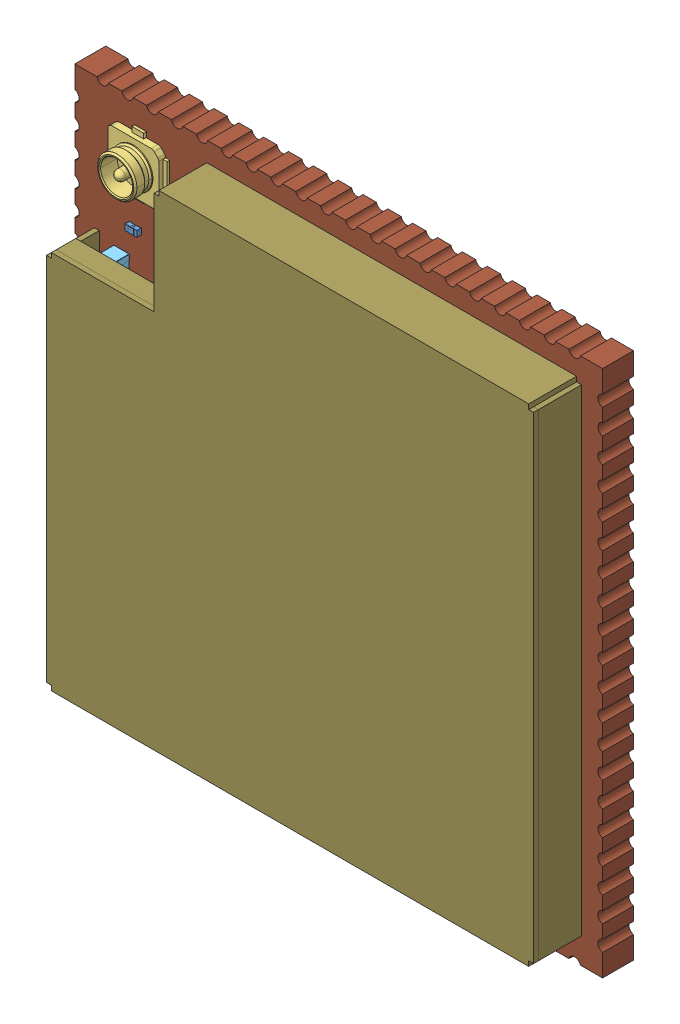
SolidWorks assembly 装配体1, configuration 默认. Lengths in mm.
Overall size (26.97 26.97 4.04).
150 component instances, 12 part files, 3 mates.
Components (placement in the parent):
- 3D_ESP32-P4-Core_2025-12-02-1: 3D_ESP32-P4-Core_2025-12-02 [默认] at (-120.883 -11.4499 -1.4231) size (26.97 26.97 2.85)
  - 3D_ESP32-P4-Core_2025-12-02.step-1: 3D_ESP32-P4-Core_2025-12-02.step [默认] at origin size (26.97 26.97 2.85)
    - R1~R0201~R0201_L0.6-W0.3-H0.3~E7ic.step-1: R1~R0201~R0201_L0.6-W0.3-H0.3~E7ic.step [默认] at (21.717 19.558 1.5862) x (0 -1 0) z (0 0 1) size (0.6 0.3 0.24)
      - R0201~R0201_L0.6-W0.3-H0.3~E7ic.step-1: R0201~R0201_L0.6-W0.3-H0.3~E7ic.step [默认] at origin size (0.6 0.3 0.24)
    - R1~R0201~R0201_L0.6-W0.3-H0.3~E7ic.step-2: R1~R0201~R0201_L0.6-W0.3-H0.3~E7ic.step [默认] at (21.463 20.7645 1.5862) size (0.6 0.3 0.24)
      - R0201~R0201_L0.6-W0.3-H0.3~E7ic.step-1: R0201~R0201_L0.6-W0.3-H0.3~E7ic.step [默认] at origin size (0.6 0.3 0.24)
    - R1~R0201~R0201_L0.6-W0.3-H0.3~E7ic.step-3: R1~R0201~R0201_L0.6-W0.3-H0.3~E7ic.step [默认] at (20.193 4.064 1.5862) x (0 -1 0) z (0 0 1) size (0.6 0.3 0.24)
      - R0201~R0201_L0.6-W0.3-H0.3~E7ic.step-1: R0201~R0201_L0.6-W0.3-H0.3~E7ic.step [默认] at origin size (0.6 0.3 0.24)
    - R1~R0201~R0201_L0.6-W0.3-H0.3~E7ic.step-4: R1~R0201~R0201_L0.6-W0.3-H0.3~E7ic.step [默认] at (14.351 4.1275 1.5862) x (0 -1 0) z (0 0 1) size (0.6 0.3 0.24)
      - R0201~R0201_L0.6-W0.3-H0.3~E7ic.step-1: R0201~R0201_L0.6-W0.3-H0.3~E7ic.step [默认] at origin size (0.6 0.3 0.24)
    - R1~R0201~R0201_L0.6-W0.3-H0.3~E7ic.step-5: R1~R0201~R0201_L0.6-W0.3-H0.3~E7ic.step [默认] at (9.652 15.748 1.5862) size (0.6 0.3 0.24)
      - R0201~R0201_L0.6-W0.3-H0.3~E7ic.step-1: R0201~R0201_L0.6-W0.3-H0.3~E7ic.step [默认] at origin size (0.6 0.3 0.24)
    - R1~R0201~R0201_L0.6-W0.3-H0.3~E7ic.step-6: R1~R0201~R0201_L0.6-W0.3-H0.3~E7ic.step [默认] at (9.652 14.859 1.5862) size (0.6 0.3 0.24)
      - R0201~R0201_L0.6-W0.3-H0.3~E7ic.step-1: R0201~R0201_L0.6-W0.3-H0.3~E7ic.step [默认] at origin size (0.6 0.3 0.24)
    - R1~R0201~R0201_L0.6-W0.3-H0.3~E7ic.step-7: R1~R0201~R0201_L0.6-W0.3-H0.3~E7ic.step [默认] at (9.652 13.97 1.5862) size (0.6 0.3 0.24)
      - R0201~R0201_L0.6-W0.3-H0.3~E7ic.step-1: R0201~R0201_L0.6-W0.3-H0.3~E7ic.step [默认] at origin size (0.6 0.3 0.24)
    - R1~R0201~R0201_L0.6-W0.3-H0.3~E7ic.step-8: R1~R0201~R0201_L0.6-W0.3-H0.3~E7ic.step [默认] at (9.652 13.081 1.5862) size (0.6 0.3 0.24)
      - R0201~R0201_L0.6-W0.3-H0.3~E7ic.step-1: R0201~R0201_L0.6-W0.3-H0.3~E7ic.step [默认] at origin size (0.6 0.3 0.24)
    - R1~R0201~R0201_L0.6-W0.3-H0.3~E7ic.step-9: R1~R0201~R0201_L0.6-W0.3-H0.3~E7ic.step [默认] at (10.033 9.144 1.5862) x (0 -1 0) z (0 0 1) size (0.6 0.3 0.24)
      - R0201~R0201_L0.6-W0.3-H0.3~E7ic.step-1: R0201~R0201_L0.6-W0.3-H0.3~E7ic.step [默认] at origin size (0.6 0.3 0.24)
    - R1~R0201~R0201_L0.6-W0.3-H0.3~E7ic.step-10: R1~R0201~R0201_L0.6-W0.3-H0.3~E7ic.step [默认] at (9.144 9.144 1.5862) x (0 -1 0) z (0 0 1) size (0.6 0.3 0.24)
      - R0201~R0201_L0.6-W0.3-H0.3~E7ic.step-1: R0201~R0201_L0.6-W0.3-H0.3~E7ic.step [默认] at origin size (0.6 0.3 0.24)
    - R1~R0201~R0201_L0.6-W0.3-H0.3~E7ic.step-11: R1~R0201~R0201_L0.6-W0.3-H0.3~E7ic.step [默认] at (7.239 7.62 1.5862) x (0 -1 0) z (0 0 1) size (0.6 0.3 0.24)
      - R0201~R0201_L0.6-W0.3-H0.3~E7ic.step-1: R0201~R0201_L0.6-W0.3-H0.3~E7ic.step [默认] at origin size (0.6 0.3 0.24)
    - R1~R0201~R0201_L0.6-W0.3-H0.3~E7ic.step-12: R1~R0201~R0201_L0.6-W0.3-H0.3~E7ic.step [默认] at (22.6695 5.5245 1.5862) size (0.6 0.3 0.24)
      - R0201~R0201_L0.6-W0.3-H0.3~E7ic.step-1: R0201~R0201_L0.6-W0.3-H0.3~E7ic.step [默认] at origin size (0.6 0.3 0.24)
    - R1~R0201~R0201_L0.6-W0.3-H0.3~E7ic.step-13: R1~R0201~R0201_L0.6-W0.3-H0.3~E7ic.step [默认] at (24.0665 6.0325 1.5862) x (-1 0 0) z (0 0 1) size (0.6 0.3 0.24)
      - R0201~R0201_L0.6-W0.3-H0.3~E7ic.step-1: R0201~R0201_L0.6-W0.3-H0.3~E7ic.step [默认] at origin size (0.6 0.3 0.24)
    - R1~R0201~R0201_L0.6-W0.3-H0.3~E7ic.step-14: R1~R0201~R0201_L0.6-W0.3-H0.3~E7ic.step [默认] at (3.1115 21.2725 1.5862) size (0.6 0.3 0.24)
      - R0201~R0201_L0.6-W0.3-H0.3~E7ic.step-1: R0201~R0201_L0.6-W0.3-H0.3~E7ic.step [默认] at origin size (0.6 0.3 0.24)
    - R1~R0201~R0201_L0.6-W0.3-H0.3~E7ic.step-15: R1~R0201~R0201_L0.6-W0.3-H0.3~E7ic.step [默认] at (10.3505 5.9055 1.5862) x (0 1 0) z (0 0 1) size (0.6 0.3 0.24)
      - R0201~R0201_L0.6-W0.3-H0.3~E7ic.step-1: R0201~R0201_L0.6-W0.3-H0.3~E7ic.step [默认] at origin size (0.6 0.3 0.24)
    - R1~R0201~R0201_L0.6-W0.3-H0.3~E7ic.step-16: R1~R0201~R0201_L0.6-W0.3-H0.3~E7ic.step [默认] at (5.3975 7.493 1.5862) x (-1 0 0) z (0 0 1) size (0.6 0.3 0.24)
      - R0201~R0201_L0.6-W0.3-H0.3~E7ic.step-1: R0201~R0201_L0.6-W0.3-H0.3~E7ic.step [默认] at origin size (0.6 0.3 0.24)
    - R1~R0201~R0201_L0.6-W0.3-H0.3~E7ic.step-17: R1~R0201~R0201_L0.6-W0.3-H0.3~E7ic.step [默认] at (24.638 20.7645 1.5862) x (0 -1 0) z (0 0 1) size (0.6 0.3 0.24)
      - R0201~R0201_L0.6-W0.3-H0.3~E7ic.step-1: R0201~R0201_L0.6-W0.3-H0.3~E7ic.step [默认] at origin size (0.6 0.3 0.24)
    - L2~L0201~L0201-RD~E7ic.step-1: L2~L0201~L0201-RD~E7ic.step [默认] at (3.302 15.24 1.5862) x (0.707107 -0.707107 0) z (0 0 1) size (0.6 0.3 0.3)
      - L0201~L0201-RD~E7ic.step-1: L0201~L0201-RD~E7ic.step [默认] at origin size (0.6 0.3 0.3)
    - L2~L0201~L0201-RD~E7ic.step-2: L2~L0201~L0201-RD~E7ic.step [默认] at (7.6835 16.637 1.5862) x (0 1 0) z (0 0 1) size (0.6 0.3 0.3)
      - L0201~L0201-RD~E7ic.step-1: L0201~L0201-RD~E7ic.step [默认] at origin size (0.6 0.3 0.3)
    - L2~L0201~L0201-RD~E7ic.step-3: L2~L0201~L0201-RD~E7ic.step [默认] at (4.5085 17.78 1.5862) x (-0.707107 0.707107 0) z (0 0 1) size (0.6 0.3 0.3)
      - L0201~L0201-RD~E7ic.step-1: L0201~L0201-RD~E7ic.step [默认] at origin size (0.6 0.3 0.3)
    - RF1~ANT-SMD_73412-0110~ANT-SMD_73412-0110~E7ic.step-1: RF1~ANT-SMD_73412-0110~ANT-SMD_73412-0110~E7ic.step [默认] at (3.3655 24.257 1.5862) size (3 3.12 1.26)
      - ANT-SMD_73412-0110~ANT-SMD_73412-0110~E7ic.step-1: ANT-SMD_73412-0110~ANT-SMD_73412-0110~E7ic.step [默认] at origin size (3 3.12 1.26)
    - C2~C0201~C0201_L0.6-W0.3-H0.3~E7ic.step-1: C2~C0201~C0201_L0.6-W0.3-H0.3~E7ic.step [默认] at (16.4465 20.1295 1.5862) x (0 -1 0) z (0 0 1) size (0.6 0.3 0.3)
      - C0201~C0201_L0.6-W0.3-H0.3~E7ic.step-1: C0201~C0201_L0.6-W0.3-H0.3~E7ic.step [默认] at origin size (0.6 0.3 0.3)
    - C2~C0201~C0201_L0.6-W0.3-H0.3~E7ic.step-2: C2~C0201~C0201_L0.6-W0.3-H0.3~E7ic.step [默认] at (17.653 19.558 1.5862) size (0.6 0.3 0.3)
      - C0201~C0201_L0.6-W0.3-H0.3~E7ic.step-1: C0201~C0201_L0.6-W0.3-H0.3~E7ic.step [默认] at origin size (0.6 0.3 0.3)
    - C2~C0201~C0201_L0.6-W0.3-H0.3~E7ic.step-3: C2~C0201~C0201_L0.6-W0.3-H0.3~E7ic.step [默认] at (13.5255 19.8755 1.5862) x (0 -1 0) z (0 0 1) size (0.6 0.3 0.3)
      - C0201~C0201_L0.6-W0.3-H0.3~E7ic.step-1: C0201~C0201_L0.6-W0.3-H0.3~E7ic.step [默认] at origin size (0.6 0.3 0.3)
    - C2~C0201~C0201_L0.6-W0.3-H0.3~E7ic.step-4: C2~C0201~C0201_L0.6-W0.3-H0.3~E7ic.step [默认] at (19.177 19.558 1.5862) size (0.6 0.3 0.3)
      - C0201~C0201_L0.6-W0.3-H0.3~E7ic.step-1: C0201~C0201_L0.6-W0.3-H0.3~E7ic.step [默认] at origin size (0.6 0.3 0.3)
    - C2~C0201~C0201_L0.6-W0.3-H0.3~E7ic.step-5: C2~C0201~C0201_L0.6-W0.3-H0.3~E7ic.step [默认] at (12.6365 19.8755 1.5862) x (0 -1 0) z (0 0 1) size (0.6 0.3 0.3)
      - C0201~C0201_L0.6-W0.3-H0.3~E7ic.step-1: C0201~C0201_L0.6-W0.3-H0.3~E7ic.step [默认] at origin size (0.6 0.3 0.3)
    - C2~C0201~C0201_L0.6-W0.3-H0.3~E7ic.step-6: C2~C0201~C0201_L0.6-W0.3-H0.3~E7ic.step [默认] at (24.511 15.748 1.5862) x (-1 0 0) z (0 0 1) size (0.6 0.3 0.3)
      - C0201~C0201_L0.6-W0.3-H0.3~E7ic.step-1: C0201~C0201_L0.6-W0.3-H0.3~E7ic.step [默认] at origin size (0.6 0.3 0.3)
    - C2~C0201~C0201_L0.6-W0.3-H0.3~E7ic.step-7: C2~C0201~C0201_L0.6-W0.3-H0.3~E7ic.step [默认] at (24.511 13.97 1.5862) x (-1 0 0) z (0 0 1) size (0.6 0.3 0.3)
      - C0201~C0201_L0.6-W0.3-H0.3~E7ic.step-1: C0201~C0201_L0.6-W0.3-H0.3~E7ic.step [默认] at origin size (0.6 0.3 0.3)
    - C2~C0201~C0201_L0.6-W0.3-H0.3~E7ic.step-8: C2~C0201~C0201_L0.6-W0.3-H0.3~E7ic.step [默认] at (24.511 14.859 1.5862) x (-1 0 0) z (0 0 1) size (0.6 0.3 0.3)
      - C0201~C0201_L0.6-W0.3-H0.3~E7ic.step-1: C0201~C0201_L0.6-W0.3-H0.3~E7ic.step [默认] at origin size (0.6 0.3 0.3)
    - C2~C0201~C0201_L0.6-W0.3-H0.3~E7ic.step-9: C2~C0201~C0201_L0.6-W0.3-H0.3~E7ic.step [默认] at (9.906 11.8745 1.5862) x (0 1 0) z (0 0 1) size (0.6 0.3 0.3)
      - C0201~C0201_L0.6-W0.3-H0.3~E7ic.step-1: C0201~C0201_L0.6-W0.3-H0.3~E7ic.step [默认] at origin size (0.6 0.3 0.3)
    - C2~C0201~C0201_L0.6-W0.3-H0.3~E7ic.step-10: C2~C0201~C0201_L0.6-W0.3-H0.3~E7ic.step [默认] at (24.511 10.414 1.5862) x (-1 0 0) z (0 0 1) size (0.6 0.3 0.3)
      - C0201~C0201_L0.6-W0.3-H0.3~E7ic.step-1: C0201~C0201_L0.6-W0.3-H0.3~E7ic.step [默认] at origin size (0.6 0.3 0.3)
    - C2~C0201~C0201_L0.6-W0.3-H0.3~E7ic.step-11: C2~C0201~C0201_L0.6-W0.3-H0.3~E7ic.step [默认] at (24.511 11.303 1.5862) x (-1 0 0) z (0 0 1) size (0.6 0.3 0.3)
      - C0201~C0201_L0.6-W0.3-H0.3~E7ic.step-1: C0201~C0201_L0.6-W0.3-H0.3~E7ic.step [默认] at origin size (0.6 0.3 0.3)
    - C2~C0201~C0201_L0.6-W0.3-H0.3~E7ic.step-12: C2~C0201~C0201_L0.6-W0.3-H0.3~E7ic.step [默认] at (24.511 12.192 1.5862) x (-1 0 0) z (0 0 1) size (0.6 0.3 0.3)
      - C0201~C0201_L0.6-W0.3-H0.3~E7ic.step-1: C0201~C0201_L0.6-W0.3-H0.3~E7ic.step [默认] at origin size (0.6 0.3 0.3)
    - C2~C0201~C0201_L0.6-W0.3-H0.3~E7ic.step-13: C2~C0201~C0201_L0.6-W0.3-H0.3~E7ic.step [默认] at (24.511 13.081 1.5862) x (-1 0 0) z (0 0 1) size (0.6 0.3 0.3)
      - C0201~C0201_L0.6-W0.3-H0.3~E7ic.step-1: C0201~C0201_L0.6-W0.3-H0.3~E7ic.step [默认] at origin size (0.6 0.3 0.3)
    - C2~C0201~C0201_L0.6-W0.3-H0.3~E7ic.step-14: C2~C0201~C0201_L0.6-W0.3-H0.3~E7ic.step [默认] at (24.511 9.525 1.5862) x (-1 0 0) z (0 0 1) size (0.6 0.3 0.3)
      - C0201~C0201_L0.6-W0.3-H0.3~E7ic.step-1: C0201~C0201_L0.6-W0.3-H0.3~E7ic.step [默认] at origin size (0.6 0.3 0.3)
    - C2~C0201~C0201_L0.6-W0.3-H0.3~E7ic.step-15: C2~C0201~C0201_L0.6-W0.3-H0.3~E7ic.step [默认] at (9.144 7.6835 1.5862) x (0 1 0) z (0 0 1) size (0.6 0.3 0.3)
      - C0201~C0201_L0.6-W0.3-H0.3~E7ic.step-1: C0201~C0201_L0.6-W0.3-H0.3~E7ic.step [默认] at origin size (0.6 0.3 0.3)
    - C2~C0201~C0201_L0.6-W0.3-H0.3~E7ic.step-16: C2~C0201~C0201_L0.6-W0.3-H0.3~E7ic.step [默认] at (24.511 8.636 1.5862) x (-1 0 0) z (0 0 1) size (0.6 0.3 0.3)
      - C0201~C0201_L0.6-W0.3-H0.3~E7ic.step-1: C0201~C0201_L0.6-W0.3-H0.3~E7ic.step [默认] at origin size (0.6 0.3 0.3)
    - C2~C0201~C0201_L0.6-W0.3-H0.3~E7ic.step-17: C2~C0201~C0201_L0.6-W0.3-H0.3~E7ic.step [默认] at (24.511 7.747 1.5862) x (-1 0 0) z (0 0 1) size (0.6 0.3 0.3)
      - C0201~C0201_L0.6-W0.3-H0.3~E7ic.step-1: C0201~C0201_L0.6-W0.3-H0.3~E7ic.step [默认] at origin size (0.6 0.3 0.3)
    - C2~C0201~C0201_L0.6-W0.3-H0.3~E7ic.step-18: C2~C0201~C0201_L0.6-W0.3-H0.3~E7ic.step [默认] at (10.0965 7.493 1.5862) x (0 -1 0) z (0 0 1) size (0.6 0.3 0.3)
      - C0201~C0201_L0.6-W0.3-H0.3~E7ic.step-1: C0201~C0201_L0.6-W0.3-H0.3~E7ic.step [默认] at origin size (0.6 0.3 0.3)
    - C2~C0201~C0201_L0.6-W0.3-H0.3~E7ic.step-19: C2~C0201~C0201_L0.6-W0.3-H0.3~E7ic.step [默认] at (12.5095 4.191 1.5862) x (0 1 0) z (0 0 1) size (0.6 0.3 0.3)
      - C0201~C0201_L0.6-W0.3-H0.3~E7ic.step-1: C0201~C0201_L0.6-W0.3-H0.3~E7ic.step [默认] at origin size (0.6 0.3 0.3)
    - C2~C0201~C0201_L0.6-W0.3-H0.3~E7ic.step-20: C2~C0201~C0201_L0.6-W0.3-H0.3~E7ic.step [默认] at (13.462 4.191 1.5862) x (0 1 0) z (0 0 1) size (0.6 0.3 0.3)
      - C0201~C0201_L0.6-W0.3-H0.3~E7ic.step-1: C0201~C0201_L0.6-W0.3-H0.3~E7ic.step [默认] at origin size (0.6 0.3 0.3)
    - C2~C0201~C0201_L0.6-W0.3-H0.3~E7ic.step-21: C2~C0201~C0201_L0.6-W0.3-H0.3~E7ic.step [默认] at (21.3995 4.064 1.5862) x (0 1 0) z (0 0 1) size (0.6 0.3 0.3)
      - C0201~C0201_L0.6-W0.3-H0.3~E7ic.step-1: C0201~C0201_L0.6-W0.3-H0.3~E7ic.step [默认] at origin size (0.6 0.3 0.3)
    - C2~C0201~C0201_L0.6-W0.3-H0.3~E7ic.step-22: C2~C0201~C0201_L0.6-W0.3-H0.3~E7ic.step [默认] at (22.352 4.064 1.5862) x (0 1 0) z (0 0 1) size (0.6 0.3 0.3)
      - C0201~C0201_L0.6-W0.3-H0.3~E7ic.step-1: C0201~C0201_L0.6-W0.3-H0.3~E7ic.step [默认] at origin size (0.6 0.3 0.3)
    - C2~C0201~C0201_L0.6-W0.3-H0.3~E7ic.step-23: C2~C0201~C0201_L0.6-W0.3-H0.3~E7ic.step [默认] at (4.6355 16.383 1.5862) x (0.707107 0.707107 0) z (0 0 1) size (0.6 0.3 0.3)
      - C0201~C0201_L0.6-W0.3-H0.3~E7ic.step-1: C0201~C0201_L0.6-W0.3-H0.3~E7ic.step [默认] at origin size (0.6 0.3 0.3)
    - C2~C0201~C0201_L0.6-W0.3-H0.3~E7ic.step-24: C2~C0201~C0201_L0.6-W0.3-H0.3~E7ic.step [默认] at (3.937 18.8595 1.5862) x (-0.707107 -0.707107 0) z (0 0 1) size (0.6 0.3 0.3)
      - C0201~C0201_L0.6-W0.3-H0.3~E7ic.step-1: C0201~C0201_L0.6-W0.3-H0.3~E7ic.step [默认] at origin size (0.6 0.3 0.3)
    - C2~C0201~C0201_L0.6-W0.3-H0.3~E7ic.step-25: C2~C0201~C0201_L0.6-W0.3-H0.3~E7ic.step [默认] at (6.731 16.637 1.5862) x (0 -1 0) z (0 0 1) size (0.6 0.3 0.3)
      - C0201~C0201_L0.6-W0.3-H0.3~E7ic.step-1: C0201~C0201_L0.6-W0.3-H0.3~E7ic.step [默认] at origin size (0.6 0.3 0.3)
    - C2~C0201~C0201_L0.6-W0.3-H0.3~E7ic.step-26: C2~C0201~C0201_L0.6-W0.3-H0.3~E7ic.step [默认] at (5.842 16.637 1.5862) x (0 -1 0) z (0 0 1) size (0.6 0.3 0.3)
      - C0201~C0201_L0.6-W0.3-H0.3~E7ic.step-1: C0201~C0201_L0.6-W0.3-H0.3~E7ic.step [默认] at origin size (0.6 0.3 0.3)
    - C2~C0201~C0201_L0.6-W0.3-H0.3~E7ic.step-27: C2~C0201~C0201_L0.6-W0.3-H0.3~E7ic.step [默认] at (2.4765 17.2085 1.5862) size (0.6 0.3 0.3)
      - C0201~C0201_L0.6-W0.3-H0.3~E7ic.step-1: C0201~C0201_L0.6-W0.3-H0.3~E7ic.step [默认] at origin size (0.6 0.3 0.3)
    - C2~C0201~C0201_L0.6-W0.3-H0.3~E7ic.step-28: C2~C0201~C0201_L0.6-W0.3-H0.3~E7ic.step [默认] at (2.413 14.351 1.5862) x (0.707107 0.707107 0) z (0 0 1) size (0.6 0.3 0.3)
      - C0201~C0201_L0.6-W0.3-H0.3~E7ic.step-1: C0201~C0201_L0.6-W0.3-H0.3~E7ic.step [默认] at origin size (0.6 0.3 0.3)
    - C2~C0201~C0201_L0.6-W0.3-H0.3~E7ic.step-29: C2~C0201~C0201_L0.6-W0.3-H0.3~E7ic.step [默认] at (8.1915 8.636 1.5862) x (0 1 0) z (0 0 1) size (0.6 0.3 0.3)
      - C0201~C0201_L0.6-W0.3-H0.3~E7ic.step-1: C0201~C0201_L0.6-W0.3-H0.3~E7ic.step [默认] at origin size (0.6 0.3 0.3)
    - C2~C0201~C0201_L0.6-W0.3-H0.3~E7ic.step-30: C2~C0201~C0201_L0.6-W0.3-H0.3~E7ic.step [默认] at (17.4079 4.7102 1.5862) size (0.6 0.3 0.3)
      - C0201~C0201_L0.6-W0.3-H0.3~E7ic.step-1: C0201~C0201_L0.6-W0.3-H0.3~E7ic.step [默认] at origin size (0.6 0.3 0.3)
    - C2~C0201~C0201_L0.6-W0.3-H0.3~E7ic.step-31: C2~C0201~C0201_L0.6-W0.3-H0.3~E7ic.step [默认] at (17.399 3.7465 1.5862) size (0.6 0.3 0.3)
      - C0201~C0201_L0.6-W0.3-H0.3~E7ic.step-1: C0201~C0201_L0.6-W0.3-H0.3~E7ic.step [默认] at origin size (0.6 0.3 0.3)
    - C2~C0201~C0201_L0.6-W0.3-H0.3~E7ic.step-32: C2~C0201~C0201_L0.6-W0.3-H0.3~E7ic.step [默认] at (2.4765 16.3195 1.5862) size (0.6 0.3 0.3)
      - C0201~C0201_L0.6-W0.3-H0.3~E7ic.step-1: C0201~C0201_L0.6-W0.3-H0.3~E7ic.step [默认] at origin size (0.6 0.3 0.3)
    - C2~C0201~C0201_L0.6-W0.3-H0.3~E7ic.step-33: C2~C0201~C0201_L0.6-W0.3-H0.3~E7ic.step [默认] at (12.3825 23.5585 1.5862) x (0 1 0) z (0 0 1) size (0.6 0.3 0.3)
      - C0201~C0201_L0.6-W0.3-H0.3~E7ic.step-1: C0201~C0201_L0.6-W0.3-H0.3~E7ic.step [默认] at origin size (0.6 0.3 0.3)
    - C2~C0201~C0201_L0.6-W0.3-H0.3~E7ic.step-34: C2~C0201~C0201_L0.6-W0.3-H0.3~E7ic.step [默认] at (16.1925 23.0505 1.5862) x (0 -1 0) z (0 0 1) size (0.6 0.3 0.3)
      - C0201~C0201_L0.6-W0.3-H0.3~E7ic.step-1: C0201~C0201_L0.6-W0.3-H0.3~E7ic.step [默认] at origin size (0.6 0.3 0.3)
    - C2~C0201~C0201_L0.6-W0.3-H0.3~E7ic.step-35: C2~C0201~C0201_L0.6-W0.3-H0.3~E7ic.step [默认] at (7.8105 22.098 1.5862) x (-1 0 0) z (0 0 1) size (0.6 0.3 0.3)
      - C0201~C0201_L0.6-W0.3-H0.3~E7ic.step-1: C0201~C0201_L0.6-W0.3-H0.3~E7ic.step [默认] at origin size (0.6 0.3 0.3)
    - C2~C0201~C0201_L0.6-W0.3-H0.3~E7ic.step-36: C2~C0201~C0201_L0.6-W0.3-H0.3~E7ic.step [默认] at (5.461 20.828 1.5862) x (0 -1 0) z (0 0 1) size (0.6 0.3 0.3)
      - C0201~C0201_L0.6-W0.3-H0.3~E7ic.step-1: C0201~C0201_L0.6-W0.3-H0.3~E7ic.step [默认] at origin size (0.6 0.3 0.3)
    - C2~C0201~C0201_L0.6-W0.3-H0.3~E7ic.step-37: C2~C0201~C0201_L0.6-W0.3-H0.3~E7ic.step [默认] at (21.463 21.717 1.5862) x (-1 0 0) z (0 0 1) size (0.6 0.3 0.3)
      - C0201~C0201_L0.6-W0.3-H0.3~E7ic.step-1: C0201~C0201_L0.6-W0.3-H0.3~E7ic.step [默认] at origin size (0.6 0.3 0.3)
    - C1~C0603~C0603_L1.6-W0.8-H0.8~E7ic.step-1: C1~C0603~C0603_L1.6-W0.8-H0.8~E7ic.step [默认] at (18.9865 22.5425 1.5862) size (1.6 0.8 0.8)
      - C0603~C0603_L1.6-W0.8-H0.8~E7ic.step-1: C0603~C0603_L1.6-W0.8-H0.8~E7ic.step [默认] at origin size (1.6 0.8 0.8)
    - C1~C0603~C0603_L1.6-W0.8-H0.8~E7ic.step-2: C1~C0603~C0603_L1.6-W0.8-H0.8~E7ic.step [默认] at (18.415 20.828 1.5862) size (1.6 0.8 0.8)
      - C0603~C0603_L1.6-W0.8-H0.8~E7ic.step-1: C0603~C0603_L1.6-W0.8-H0.8~E7ic.step [默认] at origin size (1.6 0.8 0.8)
    - C1~C0603~C0603_L1.6-W0.8-H0.8~E7ic.step-3: C1~C0603~C0603_L1.6-W0.8-H0.8~E7ic.step [默认] at (11.3594 20.3166 1.5862) x (0 -1 0) z (0 0 1) size (1.6 0.8 0.8)
      - C0603~C0603_L1.6-W0.8-H0.8~E7ic.step-1: C0603~C0603_L1.6-W0.8-H0.8~E7ic.step [默认] at origin size (1.6 0.8 0.8)
    - C1~C0603~C0603_L1.6-W0.8-H0.8~E7ic.step-4: C1~C0603~C0603_L1.6-W0.8-H0.8~E7ic.step [默认] at (23.749 17.018 1.5862) size (1.6 0.8 0.8)
      - C0603~C0603_L1.6-W0.8-H0.8~E7ic.step-1: C0603~C0603_L1.6-W0.8-H0.8~E7ic.step [默认] at origin size (1.6 0.8 0.8)
    - C1~C0603~C0603_L1.6-W0.8-H0.8~E7ic.step-5: C1~C0603~C0603_L1.6-W0.8-H0.8~E7ic.step [默认] at (3.1115 7.62 1.5862) size (1.6 0.8 0.8)
      - C0603~C0603_L1.6-W0.8-H0.8~E7ic.step-1: C0603~C0603_L1.6-W0.8-H0.8~E7ic.step [默认] at origin size (1.6 0.8 0.8)
    - C1~C0603~C0603_L1.6-W0.8-H0.8~E7ic.step-6: C1~C0603~C0603_L1.6-W0.8-H0.8~E7ic.step [默认] at (23.6855 3.556 1.5862) x (0 1 0) z (0 0 1) size (1.6 0.8 0.8)
      - C0603~C0603_L1.6-W0.8-H0.8~E7ic.step-1: C0603~C0603_L1.6-W0.8-H0.8~E7ic.step [默认] at origin size (1.6 0.8 0.8)
    - C1~C0603~C0603_L1.6-W0.8-H0.8~E7ic.step-7: C1~C0603~C0603_L1.6-W0.8-H0.8~E7ic.step [默认] at (2.413 19.177 1.5862) x (0 -1 0) z (0 0 1) size (1.6 0.8 0.8)
      - C0603~C0603_L1.6-W0.8-H0.8~E7ic.step-1: C0603~C0603_L1.6-W0.8-H0.8~E7ic.step [默认] at origin size (1.6 0.8 0.8)
    - C1~C0603~C0603_L1.6-W0.8-H0.8~E7ic.step-8: C1~C0603~C0603_L1.6-W0.8-H0.8~E7ic.step [默认] at (16.9545 2.413 1.5862) size (1.6 0.8 0.8)
      - C0603~C0603_L1.6-W0.8-H0.8~E7ic.step-1: C0603~C0603_L1.6-W0.8-H0.8~E7ic.step [默认] at origin size (1.6 0.8 0.8)
    - C1~C0603~C0603_L1.6-W0.8-H0.8~E7ic.step-9: C1~C0603~C0603_L1.6-W0.8-H0.8~E7ic.step [默认] at (23.749 18.669 1.5862) size (1.6 0.8 0.8)
      - C0603~C0603_L1.6-W0.8-H0.8~E7ic.step-1: C0603~C0603_L1.6-W0.8-H0.8~E7ic.step [默认] at origin size (1.6 0.8 0.8)
    - X1~CRYSTAL-SMD_4P-L2.0-W1.6-BL~CRYSTAL-SMD_4P-L2.0-W1.6-BL~E7ic.step-1: X1~CRYSTAL-SMD_4P-L2.0-W1.6-BL~CRYSTAL-SMD_4P-L2.0-W1.6-BL~E7ic.step [默认] at (7.366 20.3835 1.5862) size (2.05 1.65 0.46)
      - CRYSTAL-SMD_4P-L2.0-W1.6-BL~CRYSTAL-SMD_4P-L2.0-W1.6-BL~E7ic.step-1: CRYSTAL-SMD_4P-L2.0-W1.6-BL~CRYSTAL-SMD_4P-L2.0-W1.6-BL~E7ic.step [默认] at origin size (2.05 1.65 0.46)
    - X1~CRYSTAL-SMD_4P-L2.0-W1.6-BL~CRYSTAL-SMD_4P-L2.0-W1.6-BL~E7ic.step-2: X1~CRYSTAL-SMD_4P-L2.0-W1.6-BL~CRYSTAL-SMD_4P-L2.0-W1.6-BL~E7ic.step [默认] at (14.3039 22.743 1.5862) size (2.05 1.65 0.46)
      - CRYSTAL-SMD_4P-L2.0-W1.6-BL~CRYSTAL-SMD_4P-L2.0-W1.6-BL~E7ic.step-1: CRYSTAL-SMD_4P-L2.0-W1.6-BL~CRYSTAL-SMD_4P-L2.0-W1.6-BL~E7ic.step [默认] at origin size (2.05 1.65 0.46)
    - U5~VFQFN-32_L5.0-W5.0-P0.50-TL-EP3.7~VFQFN-32_L5.0-W5.0-P0.50-TL-EP3.7~E7ic.step-1: U5~VFQFN-32_L5.0-W5.0-P0.50-TL-EP3.7~VFQFN-32_L5.0-W5.0-P0.50-TL-EP3.7~E7ic.step [默认] at (5.4792 11.968 1.5862) x (0.707107 -0.707107 0) z (0 0 1) size (5.02 5.02 0.75)
      - VFQFN-32_L5.0-W5.0-P0.50-TL-EP3.7~VFQFN-32_L5.0-W5.0-P0.50-TL-EP3.7~E7ic.step-1: VFQFN-32_L5.0-W5.0-P0.50-TL-EP3.7~VFQFN-32_L5.0-W5.0-P0.50-TL-EP3.7~E7ic.step [默认] at origin size (5.02 5.02 0.75)
    - U3~WSON-8_L6.0-W5.0-P1.27-BL-EP~WSON-8_L6.0-W5.0-H0.7-P1.27~E7ic.step-1: U3~WSON-8_L6.0-W5.0-P1.27-BL-EP~WSON-8_L6.0-W5.0-H0.7-P1.27~E7ic.step [默认] at (6.096 4.2545 1.5862) x (0 -1 0) z (0 0 1) size (5 6.02 0.71)
      - WSON-8_L6.0-W5.0-P1.27-BL-EP~WSON-8_L6.0-W5.0-H0.7-P1.27~E7ic.step-1: WSON-8_L6.0-W5.0-P1.27-BL-EP~WSON-8_L6.0-W5.0-H0.7-P1.27~E7ic.step [默认] at origin size (5 6.02 0.71)
    - U1~SOT-563-6_L1.6-W1.2-P0.50-LS1.6-TL~SOT-563-6_L1.6-W1.2-P0.50-LS1.6-TL~E7ic.step-1: U1~SOT-563-6_L1.6-W1.2-P0.50-LS1.6-TL~SOT-563-6_L1.6-W1.2-P0.50-LS1.6-TL~E7ic.step [默认] at (23.1775 21.0185 1.5862) x (0 1 0) z (0 0 1) size (1.6 1.6 0.57)
      - SOT-563-6_L1.6-W1.2-P0.50-LS1.6-TL~SOT-563-6_L1.6-W1.2-P0.50-LS1.6-TL~E7ic.step-1: SOT-563-6_L1.6-W1.2-P0.50-LS1.6-TL~SOT-563-6_L1.6-W1.2-P0.50-LS1.6-TL~E7ic.step [默认] at origin size (1.6 1.6 0.57)
    - L1~IND-SMD_L2.0-W1.6~IND-SMD_L2.0-W1.6-H1.1~E7ic.step-1: L1~IND-SMD_L2.0-W1.6~IND-SMD_L2.0-W1.6-H1.1~E7ic.step [默认] at (23.114 23.9395 1.5862) size (2.02 1.6 1.12)
      - IND-SMD_L2.0-W1.6~IND-SMD_L2.0-W1.6-H1.1~E7ic.step-1: IND-SMD_L2.0-W1.6~IND-SMD_L2.0-W1.6-H1.1~E7ic.step [默认] at origin size (2.02 1.6 1.12)
    - Board~E7ic.step-1: Board~E7ic.step [默认] at origin size (26.97 26.97 1.59)
- ESP32屏蔽罩20250825 3D草图-1: ESP32屏蔽罩20250825 3D草图 [默认] at (-107.4203 -10.3626 2.3631) x (-1 0 0) z (0 1 0) size (24.9 2.45 24.9)
Mates (geometry in assembly coordinates):
- 重合2: coincident: plane of 3D_ESP32-P4-Core_2025-12-02-1/3D_ESP32-P4-Core_2025-12-02.step-1/Board~E7ic.step-1 through (-107.343 2.0861 0.1631) normal (0 0 1); plane of ESP32屏蔽罩20250825 3D草图-1 through (-107.4203 -22.3392 0.1631) normal (0 0 -1)
- 距离1: distance = 1 mm: plane of ESP32屏蔽罩20250825 3D草图-1 through (-119.8703 -10.1126 0.1631) normal (-1 0 0); plane of 3D_ESP32-P4-Core_2025-12-02-1/3D_ESP32-P4-Core_2025-12-02.step-1/Board~E7ic.step-1 through (-120.8703 -5.9148 -1.4231) normal (-1 0 0)
- 距离2: distance = 1 mm aligned: plane of ESP32屏蔽罩20250825 3D草图-1 through (-114.1203 14.5374 2.6131) normal (0 1 0); plane of 3D_ESP32-P4-Core_2025-12-02-1/3D_ESP32-P4-Core_2025-12-02.step-1/Board~E7ic.step-1 through (-108.9948 15.5374 -1.4231) normal (0 1 0)
